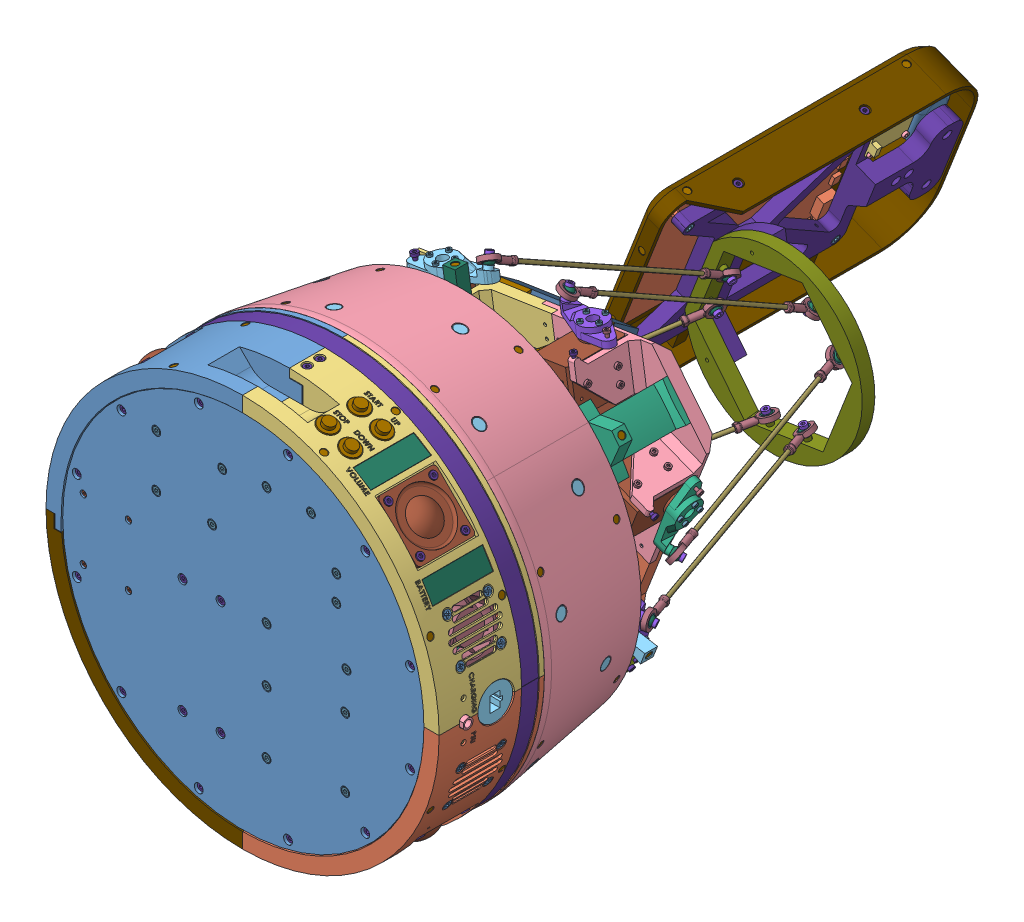
SolidWorks assembly robot orin, configuration Défaut. Lengths in mm. (continued)
Components (placement in the parent): (continued)
- base-1: base [Défaut] at (-67.3784 29.2661 438.4062) size (438.41 438.41 173) (continued)
  - magnet 5x1.6-2: magnet 5x1.6 [Défaut] at (-144.384 69.3085 585.18) x (-0.146447 -0.353553 0.92388) z (-0.92388 0.382683 0) size (5 5 1.6)
  - magnet 5x1.6-3: magnet 5x1.6 [Défaut] at (-61.581 152.1115 585.18) x (-0.353553 -0.146447 0.92388) z (-0.382683 0.92388 0) size (5 5 1.6)
  - magnet 5x1.6-4: magnet 5x1.6 [Défaut] at (55.5202 152.1115 585.18) x (-0.353553 0.146447 0.92388) z (0.382683 0.92388 0) size (5 5 1.6)
  - magnet 5x1.6-5: magnet 5x1.6 [Défaut] at (138.3232 69.3085 585.18) x (-0.146447 0.353553 0.92388) z (0.92388 0.382683 0) size (5 5 1.6)
  - magnet 5x1.6-6: magnet 5x1.6 [Défaut] at (138.3232 -47.7926 585.18) x (0.146447 0.353553 0.92388) z (0.92388 -0.382683 0) size (5 5 1.6)
  - magnet 5x1.6-7: magnet 5x1.6 [Défaut] at (55.5202 -130.5956 585.18) x (0.353553 0.146447 0.92388) z (0.382683 -0.92388 0) size (5 5 1.6)
  - magnet 5x1.6-8: magnet 5x1.6 [Défaut] at (-61.581 -130.5956 585.18) x (0.353553 -0.146447 0.92388) z (-0.382683 -0.92388 0) size (5 5 1.6)
  - magnet 5x1.6-10: magnet 5x1.6 [Défaut] at (-133.1214 -43.1275 427.3698) x (-0.137009 0.642728 -0.753744) z (-0.912505 -0.377972 -0.156434) size (5 5 1.6)
  - magnet 5x1.6-11: magnet 5x1.6 [Défaut] at (-133.1214 64.6434 427.3698) x (0.357597 0.551357 -0.753744) z (-0.912505 0.377972 -0.156434) size (5 5 1.6)
  - magnet 5x1.6-12: magnet 5x1.6 [Défaut] at (-56.9159 140.849 427.3698) x (0.642728 0.137009 -0.753744) z (-0.377972 0.912505 -0.156434) size (5 5 1.6)
  - magnet 5x1.6-13: magnet 5x1.6 [Défaut] at (50.8551 140.849 427.3698) x (0.551357 -0.357597 -0.753744) z (0.377972 0.912505 -0.156434) size (5 5 1.6)
  - magnet 5x1.6-14: magnet 5x1.6 [Défaut] at (127.0606 64.6434 427.3698) x (0.137009 -0.642728 -0.753744) z (0.912505 0.377972 -0.156434) size (5 5 1.6)
  - magnet 5x1.6-15: magnet 5x1.6 [Défaut] at (127.0606 -43.1275 427.3698) x (-0.357597 -0.551357 -0.753744) z (0.912505 -0.377972 -0.156434) size (5 5 1.6)
  - magnet 5x1.6-16: magnet 5x1.6 [Défaut] at (50.8551 -119.3331 427.3698) x (-0.642728 -0.137009 -0.753744) z (0.377972 -0.912505 -0.156434) size (5 5 1.6)
  - magnet 5x1.6-18: magnet 5x1.6 [Défaut] at (-143.3897 -47.3808 497.5426) x (-0.137009 0.642728 -0.753744) z (-0.912505 -0.377972 -0.156434) size (5 5 1.6)
  - magnet 5x1.6-19: magnet 5x1.6 [Défaut] at (-143.3897 68.8967 497.5426) x (0.357597 0.551357 -0.753744) z (-0.912505 0.377972 -0.156434) size (5 5 1.6)
  - magnet 5x1.6-20: magnet 5x1.6 [Défaut] at (-61.1691 151.1172 497.5426) x (0.642728 0.137009 -0.753744) z (-0.377972 0.912505 -0.156434) size (5 5 1.6)
  - magnet 5x1.6-21: magnet 5x1.6 [Défaut] at (55.1083 151.1172 497.5426) x (0.551357 -0.357597 -0.753744) z (0.377972 0.912505 -0.156434) size (5 5 1.6)
  - magnet 5x1.6-22: magnet 5x1.6 [Défaut] at (137.3289 68.8967 497.5426) x (0.137009 -0.642728 -0.753744) z (0.912505 0.377972 -0.156434) size (5 5 1.6)
  - magnet 5x1.6-23: magnet 5x1.6 [Défaut] at (137.3289 -47.3808 497.5426) x (-0.357597 -0.551357 -0.753744) z (0.912505 -0.377972 -0.156434) size (5 5 1.6)
  - magnet 5x1.6-24: magnet 5x1.6 [Défaut] at (55.1083 -129.6014 497.5426) x (-0.642728 -0.137009 -0.753744) z (0.377972 -0.912505 -0.156434) size (5 5 1.6)
  - magnet 5x1.6-26: magnet 5x1.6 [Défaut] at (-144.384 69.3085 528.68) x (-0.146447 -0.353553 0.92388) z (-0.92388 0.382683 0) size (5 5 1.6)
  - magnet 5x1.6-27: magnet 5x1.6 [Défaut] at (-61.581 152.1115 528.68) x (-0.353553 -0.146447 0.92388) z (-0.382683 0.92388 0) size (5 5 1.6)
  - magnet 5x1.6-28: magnet 5x1.6 [Défaut] at (55.5202 152.1115 528.68) x (-0.353553 0.146447 0.92388) z (0.382683 0.92388 0) size (5 5 1.6)
  - magnet 5x1.6-29: magnet 5x1.6 [Défaut] at (138.3232 69.3085 528.68) x (-0.146447 0.353553 0.92388) z (0.92388 0.382683 0) size (5 5 1.6)
  - magnet 5x1.6-30: magnet 5x1.6 [Défaut] at (138.3232 -47.7926 528.68) x (0.146447 0.353553 0.92388) z (0.92388 -0.382683 0) size (5 5 1.6)
  - magnet 5x1.6-31: magnet 5x1.6 [Défaut] at (55.5202 -130.5956 528.68) x (0.353553 0.146447 0.92388) z (0.382683 -0.92388 0) size (5 5 1.6)
  - magnet 5x1.6-32: magnet 5x1.6 [Défaut] at (-61.581 -130.5956 528.68) x (0.353553 -0.146447 0.92388) z (-0.382683 -0.92388 0) size (5 5 1.6)
- torso bottom orin-1: torso bottom orin [Défaut] at (-346.4088 28.5468 798.7391) x (0 0 -1) z (1 0 0) size (138.9 284.88 285.65) (flexible)
  - base gear-1: base gear [Défaut] at (-29.7845 -73.604 101.0471) size (13.91 276 276)
    - base gear 1-1: base gear 1 [Défaut] at (-37.0626 85.0813 174.9529) size (10 121.52 174.95)
    - base gear 2-1: base gear 2 [Défaut] at (-37.0626 85.0813 174.9529) size (10 174.95 121.52)
    - base gear 3-1: base gear 3 [Défaut] at (-37.0626 85.0813 174.9529) size (10 121.52 174.95)
    - base gear 4-1: base gear 4 [Défaut] at (-37.0626 85.0813 174.9529) size (13.91 174.95 121.52)
    - M3x6mm plastic-1: M3x6mm plastic [Défaut] at (-36.0626 58.0825 44.722) x (0 0 -1) z (1 0 0) size (5.5 5.5 8.3)
    - M3x6mm plastic-2: M3x6mm plastic [Défaut] at (-36.0626 215.3121 147.9541) x (0 0 -1) z (1 0 0) size (5.5 5.5 8.3)
    - M3x6mm plastic-3: M3x6mm plastic [Défaut] at (-36.0626 112.08 305.1837) x (0 0 -1) z (1 0 0) size (5.5 5.5 8.3)
    - M3x6mm plastic-4: M3x6mm plastic [Défaut] at (-36.0626 -45.1495 201.9516) x (0 0 -1) z (1 0 0) size (5.5 5.5 8.3)
  - torso bottom external-1: torso bottom external [Défaut] at (174.2366 -59.8441 326.8962) x (0 0.15099 0.988535) z (-1 0 0) size (250 250 10)
    - torso bottom external 1-1: torso bottom external 1 [Défaut] at (-39.5438 78.1885 220.0837) size (220.08 104.52 10)
    - torso bottom external 2-1: torso bottom external 2 [Défaut] at (-39.5438 78.1885 220.0837) size (165.18 170.3 10)
    - torso bottom external 3-1: torso bottom external 3 [Défaut] at (-39.5438 78.1885 220.0837) size (109.03 217.53 10)
    - M3x6mm plastic-1: M3x6mm plastic [Défaut] at (-119.0039 2.1221 229.0837) x (-1 0 0) z (0 0 -1) size (5.5 5.5 8.3)
    - M3x6mm plastic-2: M3x6mm plastic [Défaut] at (-126.2275 -4.793 229.0837) x (-1 0 0) z (0 0 -1) size (5.5 5.5 8.3)
    - M3x6mm plastic-3: M3x6mm plastic [Défaut] at (66.0616 47.4073 229.0837) x (-1 0 0) z (0 0 -1) size (5.5 5.5 8.3)
    - M3x6mm plastic-4: M3x6mm plastic [Défaut] at (75.6621 44.609 229.0837) x (-1 0 0) z (0 0 -1) size (5.5 5.5 8.3)
    - M3x6mm plastic-5: M3x6mm plastic [Défaut] at (-65.6893 185.0362 229.0837) x (-1 0 0) z (0 0 -1) size (5.5 5.5 8.3)
    - M3x6mm plastic-6: M3x6mm plastic [Défaut] at (-68.0662 194.7496 229.0837) x (-1 0 0) z (0 0 -1) size (5.5 5.5 8.3)
  - torso bottom internal orin-1: torso bottom internal orin [Défaut] at (-45.8471 11.4773 276) x (0 -0.780601 0.625029) z (-1 0 0) size (168.5 194.56 72.9)
  - torso bottom holder-1: torso bottom holder [Défaut] at (-69.831 -103.7073 307.8637) x (0 -0.780601 0.625029) z (0 0.625029 0.780601) size (29.5 23 26.69)
    - torso bottom holder-1: torso bottom holder [Défaut] at (-16.159 -8.0161 32.1209) size (29.5 22 26.69)
    - 605zz-1: 605zz [Défaut] at (5.461 -2.0161 24.075) x (0.190809 0 0.981627) z (-0.981627 0 0.190809) size (14 14 5)
    - M5 washer-1: M5 washer [Défaut] at (0.5529 -2.0161 25.029) x (0.190809 0 0.981627) z (-0.981627 0 0.190809) size (10 10 1.1)
    - M5 washer-2: M5 washer [Défaut] at (6.5408 -2.0161 23.8651) x (0.190809 0 0.981627) z (-0.981627 0 0.190809) size (10 10 1.1)
    - M5x16mm socket-1: M5x16mm socket [Défaut] at (10.0747 -2.0161 23.1782) x (-0.981627 0 0.190809) z (-0.132069 -0.72175 -0.679437) size (21 8.5 8.5)
  - torso bottom holder-2: torso bottom holder [Défaut] at (-69.831 96.6643 359.8209) x (0 0.931592 0.363506) z (0 0.363506 -0.931592) size (29.5 23 26.69)
    - torso bottom holder-1: torso bottom holder [Défaut] at (-16.159 -8.0161 32.1209) size (29.5 22 26.69)
    - 605zz-1: 605zz [Défaut] at (5.461 -2.0161 24.075) x (0.190809 0 0.981627) z (-0.981627 0 0.190809) size (14 14 5)
    - M5 washer-1: M5 washer [Défaut] at (0.5529 -2.0161 25.029) x (0.190809 0 0.981627) z (-0.981627 0 0.190809) size (10 10 1.1)
    - M5 washer-2: M5 washer [Défaut] at (6.5408 -2.0161 23.8651) x (0.190809 0 0.981627) z (-0.981627 0 0.190809) size (10 10 1.1)
    - M5x16mm socket-1: M5x16mm socket [Défaut] at (10.0747 -2.0161 23.1782) x (-0.981627 0 0.190809) z (-0.132069 -0.72175 -0.679437) size (21 8.5 8.5)
  - torso bottom holder-3: torso bottom holder [Défaut] at (-69.831 41.4748 160.3154) x (0 -0.15099 -0.988535) z (0 -0.988535 0.15099) size (29.5 23 26.69)
    - torso bottom holder-1: torso bottom holder [Défaut] at (-16.159 -8.0161 32.1209) size (29.5 22 26.69)
    - 605zz-1: 605zz [Défaut] at (5.461 -2.0161 24.075) x (0.190809 0 0.981627) z (-0.981627 0 0.190809) size (14 14 5)
    - M5 washer-1: M5 washer [Défaut] at (0.5529 -2.0161 25.029) x (0.190809 0 0.981627) z (-0.981627 0 0.190809) size (10 10 1.1)
    - M5 washer-2: M5 washer [Défaut] at (6.5408 -2.0161 23.8651) x (0.190809 0 0.981627) z (-0.981627 0 0.190809) size (10 10 1.1)
    - M5x16mm socket-1: M5x16mm socket [Défaut] at (10.0747 -2.0161 23.1782) x (-0.981627 0 0.190809) z (-0.132069 -0.72175 -0.679437) size (21 8.5 8.5)
  - limit switch bracket-1: limit switch bracket [Défaut] at (-45.8471 11.4773 276) x (0 -0.880348 -0.474329) z (1 0 0) size (34.42 36.22 10)
  - stewart stand-1: stewart stand [Défaut] at (-45.8471 11.4773 276) x (0 0.044764 -0.998998) z (1 0 0) size (47.84 42.37 60)
  - stewart stand-2: stewart stand [Défaut] at (-45.8471 11.4773 276) x (0 0.842775 0.538266) z (1 0 0) size (47.84 42.37 60)
  - stewart stand-3: stewart stand [Défaut] at (-45.8471 11.4773 276) x (0 -0.887539 0.460732) z (1 0 0) size (47.84 42.37 60)
  - limit switch-1: limit switch [Défaut] at (-39.8471 -56.2644 391.7135) x (0 0.880348 0.474329) z (0 0.474329 -0.880348) size (20 16.7 6)
  - slip ring (SNM220A-24)-1: slip ring (SNM220A-24) [Défaut] at (-108.3471 11.4773 276) x (0 -0.625029 -0.780601) z (1 0 0) size (44 44 66.3)
  - Jetson AGX Orin-1: Jetson AGX Orin [Défaut] at (-61.5471 21.1283 201.6572) x (0 -0.625029 -0.780601) z (1 0 0) size (111.1 110 70.95)
  - gear servo bracket-1: gear servo bracket [Défaut] at (-92.1471 -24.0072 200.3179) x (0 0.780601 -0.625029) z (1 0 0) size (80.9 110.9 63)
    - gear servo bracket-1: gear servo bracket [Défaut] at (-19.6043 81.2564 46.3) size (55 84.8 42)
    - XL430-W250-T-1: XL430-W250-T [Défaut] at (-13.6043 10.5064 84.3) x (0 -1 0) z (0 0 -1) size (28.5 46.5 36)
    - torso bottom gear-1: torso bottom gear [Metric - Spur gear 1.5M 52T 20PA 10FW ---S52N75H50L9N] at (-25.6043 10.5064 35.3) x (0 0 -1) z (0 1 0) size (23 80.9 80.9)
    - M2.5x8mm plastic-1: M2.5x8mm plastic [Défaut] at (-21.6043 -0.7436 73.3) x (1 0 0) z (0 -1 0) size (4.5 4.5 9.9)
    - M2.5x8mm plastic-2: M2.5x8mm plastic [Défaut] at (2.3957 -0.7436 73.3) x (1 0 0) z (0 -1 0) size (4.5 4.5 9.9)
    - M2.5x8mm plastic-3: M2.5x8mm plastic [Défaut] at (-21.6043 -0.7436 61.3) x (1 0 0) z (0 -1 0) size (4.5 4.5 9.9)
    - M2.5x8mm plastic-4: M2.5x8mm plastic [Défaut] at (2.3957 -0.7436 61.3) x (1 0 0) z (0 -1 0) size (4.5 4.5 9.9)
    - M2.5x8mm plastic-5: M2.5x8mm plastic [Défaut] at (-34.1043 2.5064 61.3) x (0 0 1) z (-1 0 0) size (4.5 4.5 9.9)
    - M2.5x8mm plastic-6: M2.5x8mm plastic [Défaut] at (-34.1043 18.5064 61.3) x (0 0 1) z (-1 0 0) size (4.5 4.5 9.9)
    - M2x12mm socket-1: M2x12mm socket [Défaut] at (-25.6043 18.5064 51.3) x (-0.923728 -0.383049 0) z (0 0 -1) size (3.8 3.8 13.6)
    - M2x12mm socket-2: M2x12mm socket [Défaut] at (-33.6043 10.5064 51.3) x (1 0 0) z (0 0 -1) size (3.8 3.8 13.6)
    - M2x12mm socket-3: M2x12mm socket [Défaut] at (-17.6043 10.5064 51.3) x (-0.923728 -0.383049 0) z (0 0 -1) size (3.8 3.8 13.6)
    - M2x12mm socket-4: M2x12mm socket [Défaut] at (-25.6043 2.5064 51.3) x (1 0 0) z (0 0 -1) size (3.8 3.8 13.6)
  - torso bottom magnet bracket-1: torso bottom magnet bracket [Défaut] at (-45.8471 11.4773 276) x (0 0.988535 -0.15099) z (1 0 0) size (36.32 10 10)
  - M3x12mm plastic-15: M3x12mm plastic [Défaut] at (-51.8471 69.3084 176.599) x (0 -0.394461 -0.918913) z (1 0 0) size (5.5 5.5 14.3)
  - M3x12mm plastic-16: M3x12mm plastic [Défaut] at (-51.8471 36.2516 163.7002) x (0 -0.418601 -0.90817) z (1 0 0) size (5.5 5.5 14.3)
  - M3x12mm plastic-17: M3x12mm plastic [Défaut] at (-51.8471 96.3446 353.605) x (0 -0.418601 -0.90817) z (1 0 0) size (5.5 5.5 14.3)
  - M3x12mm plastic-18: M3x12mm plastic [Défaut] at (-51.8471 68.6455 375.7837) x (0 -0.418601 -0.90817) z (1 0 0) size (5.5 5.5 14.3)
  - M3x12mm plastic-19: M3x12mm plastic [Défaut] at (-51.8471 -98.1643 310.6947) x (0 -0.418601 -0.90817) z (1 0 0) size (5.5 5.5 14.3)
  - M3x12mm plastic-20: M3x12mm plastic [Défaut] at (-51.8471 -103.5221 275.6173) x (0 -0.418601 -0.90817) z (1 0 0) size (5.5 5.5 14.3)
  - M3x12mm plastic-1: M3x12mm plastic [Défaut] at (-50.8471 -79.444 337.9118) x (-0.5 0.541291 0.676021) z (0 0.780601 -0.625029) size (5.5 5.5 14.3)
  - M3x12mm plastic-2: M3x12mm plastic [Défaut] at (-50.8471 -68.8185 351.1821) x (-0.5 0.541291 0.676021) z (0 0.780601 -0.625029) size (5.5 5.5 14.3)
  - M3x12mm plastic-3: M3x12mm plastic [Défaut] at (-50.8471 110.5552 323.7842) x (-0.5 -0.314805 0.806782) z (0 -0.931592 -0.363506) size (5.5 5.5 14.3)
  - M3x12mm plastic-4: M3x12mm plastic [Défaut] at (-50.8471 116.7348 307.9472) x (-0.5 -0.314805 0.806782) z (0 -0.931592 -0.363506) size (5.5 5.5 14.3)
  - M3x12mm plastic-5: M3x12mm plastic [Défaut] at (-50.8471 3.3207 166.3039) x (1 0 0) z (0 0.15099 0.988535) size (5.5 5.5 14.3)
  - M3x12mm plastic-6: M3x12mm plastic [Défaut] at (-50.8471 -13.4844 168.8708) x (1 0 0) z (0 0.15099 0.988535) size (5.5 5.5 14.3)
  - M5x16mm socket-1: M5x16mm socket [Défaut] at (-51.8471 -101.0124 232.1066) x (0 0.931592 0.363506) z (-1 0 0) size (21 8.5 8.5)
  - M5x16mm socket-2: M5x16mm socket [Défaut] at (-51.8471 29.7094 395.3656) x (0 -0.15099 -0.988535) z (0.874242 0.479924 -0.073304) size (21 8.5 8.5)
  - M5x16mm socket-3: M5x16mm socket [Défaut] at (-51.8471 105.7349 200.5277) x (0 -0.780601 0.625029) z (-1 0 0) size (21 8.5 8.5)
  - 605zz-1: 605zz [Défaut] at (-51.8471 -93.3501 235.0965) x (-0.5 -0.314805 0.806782) z (0 -0.931592 -0.363506) size (14 14 5)
  - 605zz-2: 605zz [Défaut] at (-51.8471 99.3145 205.6686) x (-0.5 0.541291 0.676021) z (0 0.780601 -0.625029) size (14 14 5)
  - 605zz-3: 605zz [Défaut] at (-51.8471 28.4675 387.2349) x (1 0 0) z (0 0.15099 0.988535) size (14 14 5)
  - M5 washer-1: M5 washer [Défaut] at (-51.8471 -92.3253 235.4963) x (0.785714 -0.224861 0.576273) z (0 -0.931592 -0.363506) size (10 10 1.1)
  - M5 washer-2: M5 washer [Défaut] at (-51.8471 -98.008 233.279) x (-0.5 -0.314805 0.806782) z (0 -0.931592 -0.363506) size (10 10 1.1)
  - M5 washer-3: M5 washer [Défaut] at (-51.8471 98.4558 206.3561) x (0.785714 0.386637 0.482872) z (0 0.780601 -0.625029) size (10 10 1.1)
  - M5 washer-4: M5 washer [Défaut] at (-51.8471 103.2175 202.5434) x (-0.5 0.541291 0.676021) z (0 0.780601 -0.625029) size (10 10 1.1)
  - M5 washer-5: M5 washer [Défaut] at (-51.8471 28.3014 386.1475) x (1 0 0) z (0 0.15099 0.988535) size (10 10 1.1)
  - M5 washer-6: M5 washer [Défaut] at (-51.8471 29.2224 392.1776) x (1 0 0) z (0 0.15099 0.988535) size (10 10 1.1)
  - M5x30mm socket-1: M5x30mm socket [Défaut] at (-51.8471 -7.1957 153.7478) x (0 0.15099 0.988535) z (-0.999286 0.037354 -0.005705) size (35 8.5 8.5)
  - M5x30mm socket-2: M5x30mm socket [Défaut] at (-51.8471 126.6873 320.9548) x (0 -0.931592 -0.363506) z (-0.551976 0.303113 -0.776817) size (35 8.5 8.5)
  - M5x30mm socket-3: M5x30mm socket [Défaut] at (-51.8471 -85.0597 353.2974) x (0 0.780601 -0.625029) z (0.446156 0.559373 0.698603) size (35 8.5 8.5)
  - 605zz-4: 605zz [Défaut] at (-51.8471 -6.2679 159.8224) x (1 0 0) z (0 0.15099 0.988535) size (14 14 5)
  - 605zz-5: 605zz [Défaut] at (-51.8471 116.3047 316.9035) x (1 0 0) z (0 0.931592 0.363506) size (14 14 5)
  - 605zz-6: 605zz [Défaut] at (-51.8471 -76.3599 346.3314) x (1 0 0) z (0 -0.780601 0.625029) size (14 14 5)
  - M5 washer-7: M5 washer [Défaut] at (-51.8471 -5.5129 164.7651) x (1 0 0) z (0 0.15099 0.988535) size (10 10 1.1)
  - M5 washer-8: M5 washer [Défaut] at (-51.8471 -6.434 158.735) x (1 0 0) z (0 0.15099 0.988535) size (10 10 1.1)
  - M5 washer-9: M5 washer [Défaut] at (-51.8471 120.9626 318.721) x (1 0 0) z (0 0.931592 0.363506) size (10 10 1.1)
  - M5 washer-10: M5 washer [Défaut] at (-51.8471 115.2799 316.5037) x (1 0 0) z (0 0.931592 0.363506) size (10 10 1.1)
  - M5 washer-11: M5 washer [Défaut] at (-51.8471 -80.2629 349.4566) x (1 0 0) z (0 -0.780601 0.625029) size (10 10 1.1)
  - M5 washer-12: M5 washer [Défaut] at (-51.8471 -75.5012 345.6439) x (1 0 0) z (0 -0.780601 0.625029) size (10 10 1.1)
  - M3x12mm plastic-7: M3x12mm plastic [Défaut] at (-60.8471 99.5759 322.1837) x (-1 0 0) z (0 0.363506 -0.931592) size (5.5 5.5 14.3)
  - M3x12mm plastic-8: M3x12mm plastic [Défaut] at (-68.6271 99.5759 322.1837) x (-1 0 0) z (0 0.363506 -0.931592) size (5.5 5.5 14.3)
  - M3x12mm plastic-9: M3x12mm plastic [Défaut] at (-60.8471 -72.5683 329.2038) x (1 0 0) z (0 0.625029 0.780601) size (5.5 5.5 14.3)
  - M3x12mm plastic-10: M3x12mm plastic [Défaut] at (-68.6271 -72.5683 329.2038) x (1 0 0) z (0 0.625029 0.780601) size (5.5 5.5 14.3)
  - M3x12mm plastic-11: M3x12mm plastic [Défaut] at (-60.8471 7.4243 176.6125) x (-0.887003 -0.069722 -0.45647) z (0 -0.988535 0.15099) size (5.5 5.5 14.3)
  - M3x12mm plastic-12: M3x12mm plastic [Défaut] at (-68.6271 7.4243 176.6125) x (-1 0 0) z (0 -0.988535 0.15099) size (5.5 5.5 14.3)
  - M3x12mm plastic-13: M3x12mm plastic [Défaut] at (-51.8471 -49.1494 373.7211) x (0 -0.371556 -0.928411) z (1 0 0) size (5.5 5.5 14.3)
  - M3x12mm plastic-14: M3x12mm plastic [Défaut] at (-51.8471 -36.7882 380.3812) x (0 -0.356881 -0.93415) z (1 0 0) size (5.5 5.5 14.3)
  - M2.5x12mm plastic-1: M2.5x12mm plastic [Défaut] at (-39.8471 -50.5725 381.1494) x (1 0 0) z (0 -0.474329 0.880348) size (4.5 4.5 13.9)
  - M2.5x12mm plastic-2: M2.5x12mm plastic [Défaut] at (-39.8471 -42.2092 385.6555) x (1 0 0) z (0 -0.474329 0.880348) size (4.5 4.5 13.9)
  - M5x10mm plastic-1: M5x10mm plastic [Défaut] at (-100.7471 22.4153 289.6605) x (0 0.998825 -0.048471) z (-1 0 0) size (8.5 8.5 13.5)
  - M5x10mm plastic-2: M5x10mm plastic [Défaut] at (-100.7471 -5.8221 278.6423) x (0 0.998825 -0.048471) z (-1 0 0) size (8.5 8.5 13.5)
  - M5x10mm plastic-3: M5x10mm plastic [Défaut] at (-100.7471 17.8386 259.6971) x (0 -0.426199 -0.904629) z (-1 0 0) size (8.5 8.5 13.5)
  - M2.5x30mm socket-1: M2.5x30mm socket [Défaut] at (-9.9471 -3.0224 333.0877) x (0 -0.283256 0.959044) z (-1 0 0) size (4.5 4.5 32.5)
  - M2.5x30mm socket-2: M2.5x30mm socket [Défaut] at (-9.9471 -52.3997 271.4202) x (0 0.83924 0.543761) z (-1 0 0) size (4.5 4.5 32.5)
  - M2.5x30mm socket-3: M2.5x30mm socket [Défaut] at (-27.5471 19.4156 213.9175) x (0 0.882447 0.470412) z (-1 0 0) size (4.5 4.5 32.5)
  - M2.5x30mm socket-4: M2.5x30mm socket [Défaut] at (-9.9471 68.7929 275.585) x (0 0.885018 0.465556) z (-1 0 0) size (4.5 4.5 32.5)
  - M3x12mm plastic-21: M3x12mm plastic [Défaut] at (-51.8471 -49.4699 183.8836) x (0 -0.880491 -0.474063) z (1 0 0) size (5.5 5.5 14.3)
  - M3x12mm plastic-22: M3x12mm plastic [Défaut] at (-51.8471 -55.7202 176.0775) x (0 -0.880491 -0.474063) z (1 0 0) size (5.5 5.5 14.3)
  - M3x12mm plastic-23: M3x12mm plastic [Défaut] at (-51.8471 -71.3322 188.5781) x (0 -0.880491 -0.474063) z (1 0 0) size (5.5 5.5 14.3)
  - M3x12mm plastic-24: M3x12mm plastic [Défaut] at (-51.8471 -65.0819 196.3841) x (0 -0.880491 -0.474063) z (1 0 0) size (5.5 5.5 14.3)
  - magnet 5x1.6-7: magnet 5x1.6 [Défaut] at (-40.8471 -126.0393 297.0045) x (-1 0 0) z (0 -0.988535 0.15099) size (5 5 1.6)
  - magnet 5x1.6-12: magnet 5x1.6 [Défaut] at (-40.8471 -39.0906 405.5951) x (-1 0 0) z (0 -0.363506 0.931592) size (5 5 1.6)
  - magnet 5x1.6-11: magnet 5x1.6 [Défaut] at (-40.8471 98.426 384.5906) x (-1 0 0) z (0 0.625029 0.780601) size (5 5 1.6)
  - magnet 5x1.6-10: magnet 5x1.6 [Défaut] at (-40.8471 148.9939 254.9955) x (-1 0 0) z (0 0.988535 -0.15099) size (5 5 1.6)
  - magnet 5x1.6-9: magnet 5x1.6 [Défaut] at (-40.8471 62.0451 146.4049) x (-1 0 0) z (0 0.363506 -0.931592) size (5 5 1.6)
  - magnet 5x1.6-8: magnet 5x1.6 [Défaut] at (-40.8471 -75.4714 167.4094) x (-1 0 0) z (0 -0.625029 -0.780601) size (5 5 1.6)
  - M3x12mm plastic-25: M3x12mm plastic [Défaut] at (-51.8471 120.2162 259.391) x (0 -0.471035 0.882115) z (1 0 0) size (5.5 5.5 14.3)
  - M3x12mm plastic-26: M3x12mm plastic [Défaut] at (-51.8471 130.1015 257.8811) x (0 -0.471035 0.882115) z (1 0 0) size (5.5 5.5 14.3)
- stewart-1: stewart [Défaut] at (-98.6674 22.9925 383.3519) x (-0.363506 -0.931592 0) z (0 0 1) size (270.43 245.67 405.82)
  - stewart bottom-1: stewart bottom [Défaut] at (51.9082 27.1683 257.1781) size (269.04 236.07 88.26) (flexible)
    - stewart bottom 1-1: stewart bottom 1 [Défaut] at (-78.0467 -7.0357 134.0562) size (128.45 156.06 56.5)
    - stewart bottom 2-1: stewart bottom 2 [Défaut] at (-78.0467 -7.0357 134.0562) size (158.11 109.69 56.5)
    - stewart bottom 3-1: stewart bottom 3 [Défaut] at (-78.0467 -7.0357 134.0562) size (141.45 144.8 56.5)
    - XL430-W250-T-1: XL430-W250-T [Défaut] at (3.9424 14.9098 167.3062) x (-0.5 -0.866025 0) z (0.866025 -0.5 0) size (28.5 46.5 36)
    - XL430-W250-T-2: XL430-W250-T [Défaut] at (-18.0467 52.9962 167.3062) x (1 0 0) z (0 1 0) size (28.5 46.5 36)
    - XL430-W250-T-3: XL430-W250-T [Défaut] at (-56.0576 -89.0132 167.3062) x (-0.5 -0.866025 0) z (0.866025 -0.5 0) size (28.5 46.5 36)
    - XL430-W250-T-4: XL430-W250-T [Défaut] at (-100.0359 -89.0132 167.3062) x (-0.5 0.866025 0) z (-0.866025 -0.5 0) size (28.5 46.5 36)
    - XL430-W250-T-5: XL430-W250-T [Défaut] at (-160.0359 14.9098 167.3062) x (-0.5 0.866025 0) z (-0.866025 -0.5 0) size (28.5 46.5 36)
    - XL430-W250-T-6: XL430-W250-T [Défaut] at (-138.0467 52.9962 167.3062) x (1 0 0) z (0 1 0) size (28.5 46.5 36)
    - stewart horn left M3-1: stewart horn left M3 [Défaut] at (-139.8731 -112.0132 155.3062) x (-0.476018 0.824488 -0.305985) z (0.866025 0.5 0) size (57.5 21 11.59)
    - stewart horn left M2.5-4: stewart horn left M2.5 [Défaut] at (-138.0467 98.9962 155.3062) x (0.993445 0 0.114314) z (0 -1 0) size (57.5 21 11.59)
    - stewart horn left M2.5-3: stewart horn left M2.5 [Défaut] at (43.7796 -8.0902 155.3062) x (-0.497766 -0.862156 -0.09443) z (-0.866025 0.5 0) size (57.5 21 11.59)
    - stewart horn right M3-1: stewart horn right M3 [Défaut] at (-16.2204 -112.0132 155.3062) x (0.498739 0.863841 -0.070978) z (-0.866025 0.5 0) size (57.5 21 11.59)
    - stewart horn right M2.5-2: stewart horn right M2.5 [Défaut] at (-18.0467 98.9962 155.3062) x (-0.994742 0 0.102411) z (0 -1 0) size (57.5 21 11.59)
    - stewart horn right M2.5-3: stewart horn right M2.5 [Défaut] at (-199.8731 -8.0902 155.3062) x (0.474882 -0.82252 -0.312965) z (0.866025 0.5 0) size (57.5 21 11.59)
    - USB hub stand-1: USB hub stand [Défaut] at (-132.7404 -70.3674 134.0562) x (-0.866025 -0.5 0) z (0.5 -0.866025 0) size (19 13.3 30)
    - USB hub stand-2: USB hub stand [Défaut] at (-165.7404 -13.2097 134.0562) x (-0.866025 -0.5 0) z (0.5 -0.866025 0) size (19 13.3 30)
    - USB hub stand-3: USB hub stand [Défaut] at (-5.3531 -39.1905 134.0562) x (0.866025 -0.5 0) z (0.5 0.866025 0) size (19 13.3 30)
    - USB hub stand-4: USB hub stand [Défaut] at (-38.3531 -96.3482 134.0562) x (0.866025 -0.5 0) z (0.5 0.866025 0) size (19 13.3 30)
    - Anker USB-c hub (4 ports)-1: Anker USB-c hub (4 ports) [Défaut] at (-123.9019 -60.7196 129.4897) x (-0.5 0.866025 0) z (0.496732 0.286788 -0.819152) size (96 30 21)
    - Anker USB-c hub (4 ports)-2: Anker USB-c hub (4 ports) [Défaut] at (-31.8608 -60.9106 129.2222) x (0.5 0.866025 0) z (-0.496732 0.286788 -0.819152) size (96 30 21)
    - dynamixel control-1: dynamixel control [Défaut] at (-161.0486 20.1008 190.0562) x (-0.5 -0.866025 0) z (0.866025 -0.5 0) size (36 56 13.6)
    - M3x6mm plastic-1: M3x6mm plastic [Défaut] at (-71.5467 71.3295 143.0562) x (-0.72811 0.685461 0) z (0 0 -1) size (5.5 5.5 8.3)
    - M3x6mm plastic-2: M3x6mm plastic [Défaut] at (-71.5467 62.1628 143.0562) x (-1 0 0) z (0 0 -1) size (5.5 5.5 8.3)
    - M3x6mm plastic-3: M3x6mm plastic [Défaut] at (-21.369 -47.2642 143.0562) x (-1 0 0) z (0 0 -1) size (5.5 5.5 8.3)
    - M3x6mm plastic-4: M3x6mm plastic [Défaut] at (-13.4304 -51.8475 143.0562) x (-1 0 0) z (0 0 -1) size (5.5 5.5 8.3)
    - M3x6mm plastic-5: M3x6mm plastic [Défaut] at (-141.2245 -36.0059 143.0562) x (-1 0 0) z (0 0 -1) size (5.5 5.5 8.3)
    - M3x6mm plastic-6: M3x6mm plastic [Défaut] at (-149.1631 -40.5892 143.0562) x (-1 0 0) z (0 0 -1) size (5.5 5.5 8.3)
    - M2.5x8mm plastic-1: M2.5x8mm plastic [Défaut] at (27.861 10.338 146.3062) x (-0.923728 -0.383049 0) z (0 0 -1) size (4.5 4.5 9.9)
    - M2.5x8mm plastic-2: M2.5x8mm plastic [Défaut] at (19.861 -3.5184 146.3062) x (-0.923728 -0.383049 0) z (0 0 -1) size (4.5 4.5 9.9)
    - M2.5x8mm plastic-3: M2.5x8mm plastic [Défaut] at (-10.0467 75.9962 146.3062) x (-1 0 0) z (0 0 -1) size (4.5 4.5 9.9)
    - M2.5x8mm plastic-4: M2.5x8mm plastic [Défaut] at (-26.0467 75.9962 146.3062) x (-1 0 0) z (0 0 -1) size (4.5 4.5 9.9)
    - M2.5x8mm plastic-5: M2.5x8mm plastic [Défaut] at (-130.0467 75.9962 146.3062) x (-1 0 0) z (0 0 -1) size (4.5 4.5 9.9)
    - M2.5x8mm plastic-6: M2.5x8mm plastic [Défaut] at (-146.0467 75.9962 146.3062) x (-1 0 0) z (0 0 -1) size (4.5 4.5 9.9)
    - M2.5x8mm plastic-7: M2.5x8mm plastic [Défaut] at (-183.9545 10.338 146.3062) x (-0.923728 -0.383049 0) z (0 0 -1) size (4.5 4.5 9.9)
    - M2.5x8mm plastic-8: M2.5x8mm plastic [Défaut] at (-175.9545 -3.5184 146.3062) x (-0.923728 -0.383049 0) z (0 0 -1) size (4.5 4.5 9.9)
    - M2.5x8mm plastic-9: M2.5x8mm plastic [Défaut] at (-123.9545 -93.585 146.3062) x (-1 0 0) z (0 0 -1) size (4.5 4.5 9.9)
    - M2.5x8mm plastic-10: M2.5x8mm plastic [Défaut] at (-115.9545 -107.4414 146.3062) x (-1 0 0) z (0 0 -1) size (4.5 4.5 9.9)
    - M2.5x8mm plastic-11: M2.5x8mm plastic [Défaut] at (-40.139 -107.4414 146.3062) x (-1 0 0) z (0 0 -1) size (4.5 4.5 9.9)
    - M2.5x8mm plastic-12: M2.5x8mm plastic [Défaut] at (-32.139 -93.585 146.3062) x (-0.923728 -0.383049 0) z (0 0 -1) size (4.5 4.5 9.9)
    - M2.5x8mm plastic-13: M2.5x8mm plastic [Défaut] at (-42.139 -110.9055 159.3062) x (-0.75 0.433013 -0.5) z (-0.5 -0.866025 0) size (4.5 4.5 9.9)
    - M2.5x8mm plastic-14: M2.5x8mm plastic [Défaut] at (-52.5313 -104.9055 159.3062) x (-0.75 0.433013 -0.5) z (-0.5 -0.866025 0) size (4.5 4.5 9.9)
    - M2.5x8mm plastic-15: M2.5x8mm plastic [Défaut] at (-103.5622 -104.9055 159.3062) x (0.75 0.433013 -0.5) z (0.5 -0.866025 0) size (4.5 4.5 9.9)
    - M2.5x8mm plastic-16: M2.5x8mm plastic [Défaut] at (-113.9545 -110.9055 159.3062) x (0.75 0.433013 -0.5) z (0.5 -0.866025 0) size (4.5 4.5 9.9)
    - M2.5x8mm plastic-17: M2.5x8mm plastic [Défaut] at (17.861 -6.9825 159.3062) x (-0.75 0.433013 -0.5) z (-0.5 -0.866025 0) size (4.5 4.5 9.9)
    - M2.5x8mm plastic-18: M2.5x8mm plastic [Défaut] at (7.4687 -0.9825 159.3062) x (-0.75 0.433013 -0.5) z (-0.5 -0.866025 0) size (4.5 4.5 9.9)
    - M2.5x8mm plastic-19: M2.5x8mm plastic [Défaut] at (-173.9545 -6.9825 159.3062) x (0.75 0.433013 -0.5) z (0.5 -0.866025 0) size (4.5 4.5 9.9)
    - M2.5x8mm plastic-20: M2.5x8mm plastic [Défaut] at (-163.5622 -0.9825 159.3062) x (0.75 0.433013 -0.5) z (0.5 -0.866025 0) size (4.5 4.5 9.9)
    - M2.5x8mm plastic-21: M2.5x8mm plastic [Défaut] at (-126.0467 75.9962 159.3062) x (0 0 1) z (1 0 0) size (4.5 4.5 9.9)
    - M2.5x8mm plastic-22: M2.5x8mm plastic [Défaut] at (-126.0467 63.9962 159.3062) x (0 0 1) z (1 0 0) size (4.5 4.5 9.9)
    - M2.5x8mm plastic-23: M2.5x8mm plastic [Défaut] at (-6.0467 75.9962 159.3062) x (0 0 1) z (1 0 0) size (4.5 4.5 9.9)
    - M2.5x8mm plastic-24: M2.5x8mm plastic [Défaut] at (-6.0467 63.9962 159.3062) x (0 0 1) z (1 0 0) size (4.5 4.5 9.9)
    - M2.5x8mm plastic-25: M2.5x8mm plastic [Défaut] at (19.4687 19.8021 159.3062) x (0.75 -0.433013 -0.5) z (0.5 0.866025 0) size (4.5 4.5 9.9)
    - M2.5x8mm plastic-26: M2.5x8mm plastic [Défaut] at (29.861 13.8021 159.3062) x (0.75 -0.433013 -0.5) z (0.5 0.866025 0) size (4.5 4.5 9.9)
    - M2.5x8mm plastic-27: M2.5x8mm plastic [Défaut] at (-40.5313 -84.1209 159.3062) x (0.75 -0.433013 -0.5) z (0.5 0.866025 0) size (4.5 4.5 9.9)
    - M2.5x8mm plastic-28: M2.5x8mm plastic [Défaut] at (-30.139 -90.1209 159.3062) x (-0.75 0.433013 0.5) z (0.5 0.866025 0) size (4.5 4.5 9.9)
    - M2.5x8mm plastic-29: M2.5x8mm plastic [Défaut] at (-185.9545 13.8021 159.3062) x (-0.75 -0.433013 -0.5) z (-0.5 0.866025 0) size (4.5 4.5 9.9)
    - M2.5x8mm plastic-30: M2.5x8mm plastic [Défaut] at (-175.5622 19.8021 159.3062) x (-0.75 -0.433013 -0.5) z (-0.5 0.866025 0) size (4.5 4.5 9.9)
    - M2.5x8mm plastic-31: M2.5x8mm plastic [Défaut] at (-150.0467 63.9962 159.3062) x (0 0 1) z (-1 0 0) size (4.5 4.5 9.9)
    - M2.5x8mm plastic-32: M2.5x8mm plastic [Défaut] at (-150.0467 75.9962 159.3062) x (0 0 -1) z (-1 0 0) size (4.5 4.5 9.9)
    - M2.5x8mm plastic-33: M2.5x8mm plastic [Défaut] at (-30.0467 75.9962 159.3062) x (0 0 1) z (-1 0 0) size (4.5 4.5 9.9)
    - M2.5x8mm plastic-34: M2.5x8mm plastic [Défaut] at (-30.0467 63.9962 159.3062) x (0 0 1) z (-1 0 0) size (4.5 4.5 9.9)
    - M2.5x8mm plastic-35: M2.5x8mm plastic [Défaut] at (-125.9545 -90.1209 159.3062) x (-0.75 -0.433013 -0.5) z (-0.5 0.866025 0) size (4.5 4.5 9.9)
    - M2.5x8mm plastic-36: M2.5x8mm plastic [Défaut] at (-115.5622 -84.1209 159.3062) x (-0.75 -0.433013 -0.5) z (-0.5 0.866025 0) size (4.5 4.5 9.9)
    - M2x12mm socket-1: M2x12mm socket [Défaut] at (-127.3908 -107.6332 147.6899) x (0.476467 -0.825265 -0.303179) z (-0.866025 -0.5 0) size (3.8 3.8 13.6)
    - M2x12mm socket-2: M2x12mm socket [Défaut] at (-132.4229 -98.9173 152.8583) x (-0.105513 0.182755 -0.97748) z (-0.866025 -0.5 0) size (3.8 3.8 13.6)
    - M2x12mm socket-3: M2x12mm socket [Défaut] at (-129.8387 -103.3933 162.9225) x (-0.105513 0.182755 -0.97748) z (-0.866025 -0.5 0) size (3.8 3.8 13.6)
    - M2x12mm socket-4: M2x12mm socket [Défaut] at (-124.8066 -112.1091 157.7541) x (0.476467 -0.825265 -0.303179) z (-0.866025 -0.5 0) size (3.8 3.8 13.6)
    - M2x12mm socket-5: M2x12mm socket [Défaut] at (-187.3629 -3.7585 162.9043) x (0.295978 -0.512649 -0.80597) z (-0.866025 -0.5 0) size (3.8 3.8 13.6)
    - M2x12mm socket-6: M2x12mm socket [Défaut] at (-184.8157 -8.1703 152.8025) x (-0.372959 0.645984 -0.666038) z (-0.866025 -0.5 0) size (3.8 3.8 13.6)
    - M2x12mm socket-7: M2x12mm socket [Défaut] at (-189.8666 0.5781 147.7081) x (0.295978 -0.512649 -0.80597) z (-0.866025 -0.5 0) size (3.8 3.8 13.6)
    - M2x12mm socket-8: M2x12mm socket [Défaut] at (-192.4138 4.99 157.8099) x (-0.372959 0.645984 -0.666038) z (-0.866025 -0.5 0) size (3.8 3.8 13.6)
    - M2x12mm socket-9: M2x12mm socket [Défaut] at (-138.9613 85.9962 163.2538) x (-0.769158 0 -0.639059) z (0 1 0) size (3.8 3.8 13.6)
    - M2x12mm socket-10: M2x12mm socket [Défaut] at (-137.1322 85.9962 147.3587) x (-0.769158 0 -0.639059) z (0 1 0) size (3.8 3.8 13.6)
    - M2x12mm socket-11: M2x12mm socket [Défaut] at (-130.0992 85.9962 156.2207) x (-0.769158 0 -0.639059) z (0 1 0) size (3.8 3.8 13.6)
    - M2x12mm socket-12: M2x12mm socket [Défaut] at (-145.9943 85.9962 154.3917) x (-0.769158 0 -0.639059) z (0 1 0) size (3.8 3.8 13.6)
    - M2x12mm socket-13: M2x12mm socket [Défaut] at (-26.0047 85.9962 156.1255) x (0.994742 0 -0.102411) z (0 1 0) size (3.8 3.8 13.6)
    - M2x12mm socket-14: M2x12mm socket [Défaut] at (-18.866 85.9962 147.3483) x (-0.888781 0 -0.458333) z (0 1 0) size (3.8 3.8 13.6)
    - M2x12mm socket-15: M2x12mm socket [Défaut] at (-10.0888 85.9962 154.4869) x (-0.888781 0 -0.458333) z (0 1 0) size (3.8 3.8 13.6)
    - M2x12mm socket-16: M2x12mm socket [Défaut] at (-17.2275 85.9962 163.2642) x (-0.888781 0 -0.458333) z (0 1 0) size (3.8 3.8 13.6)
    - M2x12mm socket-17: M2x12mm socket [Défaut] at (-27.1948 -105.0215 163.286) x (-0.47988 -0.831176 0.280822) z (0.866025 -0.5 0) size (3.8 3.8 13.6)
    - M2x12mm socket-18: M2x12mm socket [Défaut] at (-27.7626 -106.005 147.3264) x (-0.47988 -0.831176 0.280822) z (0.866025 -0.5 0) size (3.8 3.8 13.6)
    - M2x12mm socket-19: M2x12mm socket [Défaut] at (-31.4686 -112.424 155.874) x (-0.47988 -0.831176 0.280822) z (0.866025 -0.5 0) size (3.8 3.8 13.6)
    - M2x12mm socket-20: M2x12mm socket [Défaut] at (-23.4888 -98.6025 154.7384) x (-0.47988 -0.831176 0.280822) z (0.866025 -0.5 0) size (3.8 3.8 13.6)
    - M2x12mm socket-21: M2x12mm socket [Défaut] at (32.1435 -2.2444 163.2705) x (-0.496461 -0.859896 0.118761) z (0.866025 -0.5 0) size (3.8 3.8 13.6)
    - M2x12mm socket-22: M2x12mm socket [Défaut] at (32.899 -0.936 147.342) x (-0.496461 -0.859896 0.118761) z (0.866025 -0.5 0) size (3.8 3.8 13.6)
    - M2x12mm socket-23: M2x12mm socket [Défaut] at (28.5391 -8.4874 154.5508) x (-0.496461 -0.859896 0.118761) z (0.866025 -0.5 0) size (3.8 3.8 13.6)
    - M2x12mm socket-24: M2x12mm socket [Défaut] at (36.5034 5.3071 156.0617) x (-0.488636 -0.846342 0.211992) z (0.866025 -0.5 0) size (3.8 3.8 13.6)
    - M3x12mm plastic-1: M3x12mm plastic [Défaut] at (-0.5983 -15.9549 141.0562) x (-0.923728 -0.383049 0) z (0 0 -1) size (5.5 5.5 14.3)
    - M3x12mm plastic-2: M3x12mm plastic [Défaut] at (-8.0983 -28.9453 141.0562) x (-0.923728 -0.383049 0) z (0 0 -1) size (5.5 5.5 14.3)
    - M3x12mm plastic-3: M3x12mm plastic [Défaut] at (-33.5983 -73.1126 141.0562) x (-1 0 0) z (0 0 -1) size (5.5 5.5 14.3)
    - M3x12mm plastic-4: M3x12mm plastic [Défaut] at (-41.0983 -86.103 141.0562) x (-1 0 0) z (0 0 -1) size (5.5 5.5 14.3)
    - M3x12mm plastic-5: M3x12mm plastic [Défaut] at (-114.9952 -86.103 141.0562) x (-0.923728 -0.383049 0) z (0 0 -1) size (5.5 5.5 14.3)
    - M3x12mm plastic-6: M3x12mm plastic [Défaut] at (-122.4952 -73.1126 141.0562) x (-0.923728 -0.383049 0) z (0 0 -1) size (5.5 5.5 14.3)
    - M3x12mm plastic-7: M3x12mm plastic [Défaut] at (-147.9952 -28.9453 141.0562) x (-0.923728 -0.383049 0) z (0 0 -1) size (5.5 5.5 14.3)
    - M3x12mm plastic-8: M3x12mm plastic [Défaut] at (-155.4952 -15.9549 141.0562) x (-1 0 0) z (0 0 -1) size (5.5 5.5 14.3)
    - M2.5x8mm plastic-37: M2.5x8mm plastic [Défaut] at (-113.9545 -110.9055 183.3062) x (0.75 0.433013 -0.5) z (0.5 -0.866025 0) size (4.5 4.5 9.9)
    - M2.5x8mm plastic-38: M2.5x8mm plastic [Défaut] at (-42.139 -110.9055 183.3062) x (0.75 -0.433013 0.5) z (-0.5 -0.866025 0) size (4.5 4.5 9.9)
    - M3x12mm plastic-9: M3x12mm plastic [Défaut] at (-37.9608 -119.6687 188.0562) x (0.25 0.433013 -0.866025) z (0.866025 -0.5 0) size (5.5 5.5 14.3)
    - M3x12mm plastic-10: M3x12mm plastic [Défaut] at (-118.1327 -119.6687 188.0562) x (0.25 -0.433013 0.866025) z (-0.866025 -0.5 0) size (5.5 5.5 14.3)
    - M3x8mm plastic-6: M3x8mm plastic [Défaut] at (-33.6086 -122.1305 156.5483) x (-0.208097 -0.360435 0.909276) z (0.866025 -0.5 0) size (5.5 5.5 10.3)
    - M2.5x8mm plastic-39: M2.5x8mm plastic [Défaut] at (29.861 13.8021 183.3062) x (0.75 -0.433013 -0.5) z (0.5 0.866025 0) size (4.5 4.5 9.9)
    - M2.5x8mm plastic-40: M2.5x8mm plastic [Défaut] at (-6.0467 75.9962 183.3062) x (0 0 -1) z (1 0 0) size (4.5 4.5 9.9)
    - M2.5x8mm plastic-41: M2.5x8mm plastic [Défaut] at (-185.9545 13.8021 183.3062) x (0.75 0.433013 0.5) z (-0.5 0.866025 0) size (4.5 4.5 9.9)
    - M2.5x8mm plastic-42: M2.5x8mm plastic [Défaut] at (-150.0467 75.9962 183.3062) x (0 0 1) z (-1 0 0) size (4.5 4.5 9.9)
    - M3x8mm plastic-7: M3x8mm plastic [Défaut] at (-122.8825 -121.4418 160.661) x (0.448793 -0.777332 -0.440841) z (-0.866025 -0.5 0) size (5.5 5.5 10.3)
    - M2.5x12mm plastic-1: M2.5x12mm plastic [Défaut] at (-195.6327 14.5653 188.0562) x (0.25 -0.433013 0.866025) z (-0.866025 -0.5 0) size (4.5 4.5 13.9)
    - M2.5x12mm plastic-2: M2.5x12mm plastic [Défaut] at (-155.5467 83.9962 188.0562) x (1 0 0) z (0 1 0) size (4.5 4.5 13.9)
    - M2.5x12mm plastic-3: M2.5x12mm plastic [Défaut] at (-0.5467 83.9962 188.0562) x (1 0 0) z (0 1 0) size (4.5 4.5 13.9)
    - M2.5x12mm plastic-4: M2.5x12mm plastic [Défaut] at (39.5392 14.5653 188.0562) x (0.25 0.433013 -0.866025) z (0.866025 -0.5 0) size (4.5 4.5 13.9)
    - M2.5x8mm plastic-43: M2.5x8mm plastic [Défaut] at (-199.5233 11.3039 160.7831) x (0.356409 -0.617318 -0.701349) z (-0.866025 -0.5 0) size (4.5 4.5 9.9)
    - M2.5x8mm plastic-44: M2.5x8mm plastic [Défaut] at (-155.432 88.9962 153.3057) x (-0.891812 0 -0.452406) z (0 1 0) size (4.5 4.5 9.9)
    - M2.5x8mm plastic-45: M2.5x8mm plastic [Défaut] at (-0.6388 88.9962 153.514) x (0.993528 0 0.11359) z (0 1 0) size (4.5 4.5 9.9)
    - M2.5x8mm plastic-46: M2.5x8mm plastic [Défaut] at (43.8302 11.9975 156.9587) x (-0.496387 -0.859767 0.120004) z (0.866025 -0.5 0) size (4.5 4.5 9.9)
    - M3x8mm plastic-8: M3x8mm plastic [Défaut] at (-150.8412 50.5806 138.5562) x (0.25 0.433013 -0.866025) z (0.866025 -0.5 0) size (5.5 5.5 10.3)
